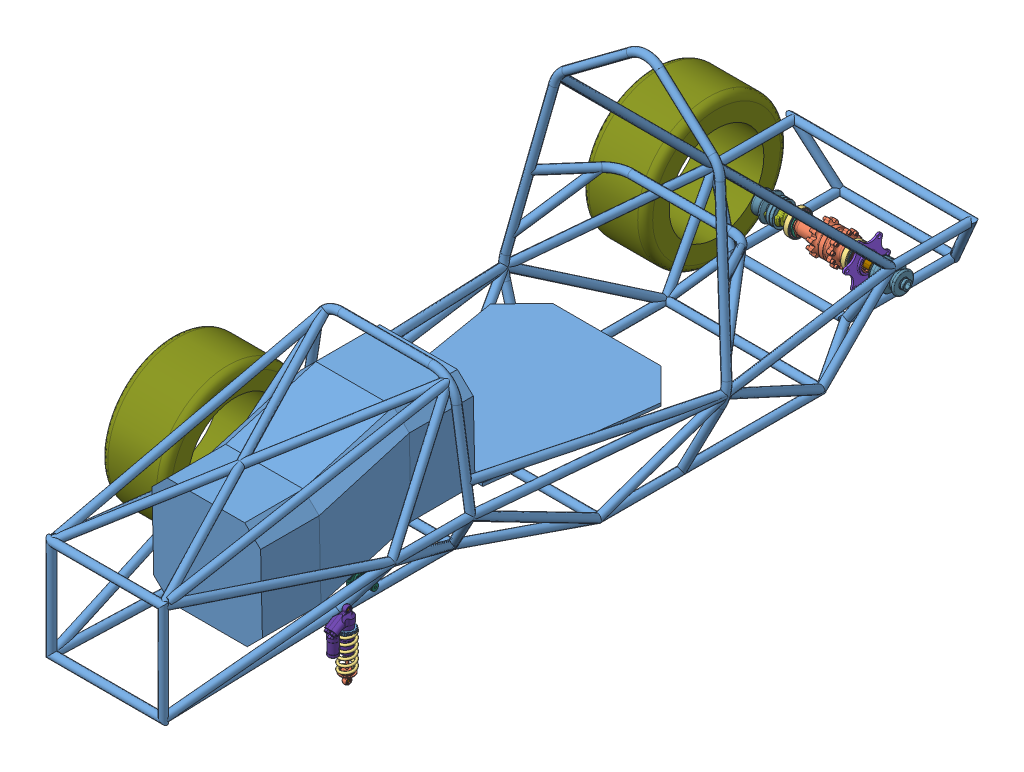
SolidWorks assembly ASSEM_Suspension24_RevA, configuration Default. Lengths in mm.
Overall size (982.83 1093.27 2583.29).
268 component instances, 21 part files, 10 mates.
Components (placement in the parent):
- 2024_Chassis_V1_RevA-1: 2024_Chassis_V1_RevA [Default<As Machined>] at origin size (743.23 992.29 2569.32)
- Differential Assembly-1: Differential Assembly [Default] at (-98.7457 437.9567 -745.2888) x (1 0 0) z (0 -0.960953 -0.276711) size (486.11 199.53 196.01)
  - Drexler Differential-1: Drexler Differential [Default] at (98.7457 177.1174 168.5551) x (0 0.999802 -0.019913) z (0 0.019913 0.999802) size (100 234.25 100)
  - SKF_32010 X-1: SKF_32010 X [Default] at (175.1207 177.1174 168.5551) x (-1 0 0) z (0 -0.454274 -0.890862) size (21.27 80 80)
    - 32010 X_or-1: 32010 X_or [Default] x (1 0 0) z (0 0 -1) size (15.5 80 80)
    - 32010 X_r-1: 32010 X_r [Default] x (1 0 0) z (0 -0.24869 -0.968583) size (15.81 10.45 7.5)
    - 32010 X_r-2: 32010 X_r [Default] x (1 0 0) z (0 -0.481754 -0.876307) size (15.81 10.45 7.5)
    - 32010 X_r-3: 32010 X_r [Default] x (1 0 0) z (0 -0.684547 -0.728969) size (15.81 10.45 7.5)
    - 32010 X_r-4: 32010 X_r [Default] x (1 0 0) z (0 -0.844328 -0.535827) size (15.81 10.45 7.5)
    - 32010 X_r-5: 32010 X_r [Default] x (1 0 0) z (0 -0.951057 -0.309017) size (15.81 10.45 7.5)
    - 32010 X_r-6: 32010 X_r [Default] x (1 0 0) z (0 -0.998027 -0.062791) size (15.81 10.45 7.5)
    - 32010 X_r-7: 32010 X_r [Default] x (1 0 0) z (0 -0.982287 0.187381) size (15.81 10.45 7.5)
    - 32010 X_r-8: 32010 X_r [Default] x (1 0 0) z (0 -0.904827 0.425779) size (15.81 10.45 7.5)
    - 32010 X_r-9: 32010 X_r [Default] x (1 0 0) z (0 -0.770513 0.637424) size (15.81 10.45 7.5)
    - 32010 X_r-10: 32010 X_r [Default] x (1 0 0) z (0 -0.587785 0.809017) size (15.81 10.45 7.5)
    - 32010 X_r-11: 32010 X_r [Default] x (1 0 0) z (0 -0.368125 0.929776) size (15.81 10.45 7.5)
    - 32010 X_r-12: 32010 X_r [Default] x (1 0 0) z (0 -0.125333 0.992115) size (15.81 10.45 7.5)
    - 32010 X_r-13: 32010 X_r [Default] x (1 0 0) z (0 0.125333 0.992115) size (15.81 10.45 7.5)
    - 32010 X_r-14: 32010 X_r [Default] x (1 0 0) z (0 0.368125 0.929776) size (15.81 10.45 7.5)
    - 32010 X_r-15: 32010 X_r [Default] x (1 0 0) z (0 0.587785 0.809017) size (15.81 10.45 7.5)
    - 32010 X_r-16: 32010 X_r [Default] x (1 0 0) z (0 0.770513 0.637424) size (15.81 10.45 7.5)
    - 32010 X_r-17: 32010 X_r [Default] x (1 0 0) z (0 0.904827 0.425779) size (15.81 10.45 7.5)
    - 32010 X_r-18: 32010 X_r [Default] x (1 0 0) z (0 0.982287 0.187381) size (15.81 10.45 7.5)
    - 32010 X_r-19: 32010 X_r [Default] x (1 0 0) z (0 0.998027 -0.062791) size (15.81 10.45 7.5)
    - 32010 X_r-20: 32010 X_r [Default] x (1 0 0) z (0 0.951057 -0.309017) size (15.81 10.45 7.5)
    - 32010 X_r-21: 32010 X_r [Default] x (1 0 0) z (0 0.844328 -0.535827) size (15.81 10.45 7.5)
    - 32010 X_r-22: 32010 X_r [Default] x (1 0 0) z (0 0.684547 -0.728969) size (15.81 10.45 7.5)
    - 32010 X_r-23: 32010 X_r [Default] x (1 0 0) z (0 0.481754 -0.876307) size (15.81 10.45 7.5)
    - 32010 X_r-24: 32010 X_r [Default] x (1 0 0) z (0 0.24869 -0.968583) size (15.81 10.45 7.5)
    - 32010 X_r-25: 32010 X_r [Default] x (1 0 0) z (0 0 -1) size (15.81 10.45 7.5)
    - 32010 X_cage-1: 32010 X_cage [Default] x (1 0 0) z (0 0 -1) size (18.02 76.15 76.15)
    - 32010 X_ir-1: 32010 X_ir [Default] x (1 0 0) z (0 0 -1) size (20 65.95 65.95)
  - SKF_32010 X-2: SKF_32010 X [Default] at (-24.8793 177.1174 168.5551) x (1 0 0) z (0 0.890912 0.454177) size (21.27 80 80)
    - 32010 X_or-1: 32010 X_or [Default] x (1 0 0) z (0 0 -1) size (15.5 80 80)
    - 32010 X_r-1: 32010 X_r [Default] x (1 0 0) z (0 -0.24869 -0.968583) size (15.81 10.45 7.5)
    - 32010 X_r-2: 32010 X_r [Default] x (1 0 0) z (0 -0.481754 -0.876307) size (15.81 10.45 7.5)
    - 32010 X_r-3: 32010 X_r [Default] x (1 0 0) z (0 -0.684547 -0.728969) size (15.81 10.45 7.5)
    - 32010 X_r-4: 32010 X_r [Default] x (1 0 0) z (0 -0.844328 -0.535827) size (15.81 10.45 7.5)
    - 32010 X_r-5: 32010 X_r [Default] x (1 0 0) z (0 -0.951057 -0.309017) size (15.81 10.45 7.5)
    - 32010 X_r-6: 32010 X_r [Default] x (1 0 0) z (0 -0.998027 -0.062791) size (15.81 10.45 7.5)
    - 32010 X_r-7: 32010 X_r [Default] x (1 0 0) z (0 -0.982287 0.187381) size (15.81 10.45 7.5)
    - 32010 X_r-8: 32010 X_r [Default] x (1 0 0) z (0 -0.904827 0.425779) size (15.81 10.45 7.5)
    - 32010 X_r-9: 32010 X_r [Default] x (1 0 0) z (0 -0.770513 0.637424) size (15.81 10.45 7.5)
    - 32010 X_r-10: 32010 X_r [Default] x (1 0 0) z (0 -0.587785 0.809017) size (15.81 10.45 7.5)
    - 32010 X_r-11: 32010 X_r [Default] x (1 0 0) z (0 -0.368125 0.929776) size (15.81 10.45 7.5)
    - 32010 X_r-12: 32010 X_r [Default] x (1 0 0) z (0 -0.125333 0.992115) size (15.81 10.45 7.5)
    - 32010 X_r-13: 32010 X_r [Default] x (1 0 0) z (0 0.125333 0.992115) size (15.81 10.45 7.5)
    - 32010 X_r-14: 32010 X_r [Default] x (1 0 0) z (0 0.368125 0.929776) size (15.81 10.45 7.5)
    - 32010 X_r-15: 32010 X_r [Default] x (1 0 0) z (0 0.587785 0.809017) size (15.81 10.45 7.5)
    - 32010 X_r-16: 32010 X_r [Default] x (1 0 0) z (0 0.770513 0.637424) size (15.81 10.45 7.5)
    - 32010 X_r-17: 32010 X_r [Default] x (1 0 0) z (0 0.904827 0.425779) size (15.81 10.45 7.5)
    - 32010 X_r-18: 32010 X_r [Default] x (1 0 0) z (0 0.982287 0.187381) size (15.81 10.45 7.5)
    - 32010 X_r-19: 32010 X_r [Default] x (1 0 0) z (0 0.998027 -0.062791) size (15.81 10.45 7.5)
    - 32010 X_r-20: 32010 X_r [Default] x (1 0 0) z (0 0.951057 -0.309017) size (15.81 10.45 7.5)
    - 32010 X_r-21: 32010 X_r [Default] x (1 0 0) z (0 0.844328 -0.535827) size (15.81 10.45 7.5)
    - 32010 X_r-22: 32010 X_r [Default] x (1 0 0) z (0 0.684547 -0.728969) size (15.81 10.45 7.5)
    - 32010 X_r-23: 32010 X_r [Default] x (1 0 0) z (0 0.481754 -0.876307) size (15.81 10.45 7.5)
    - 32010 X_r-24: 32010 X_r [Default] x (1 0 0) z (0 0.24869 -0.968583) size (15.81 10.45 7.5)
    - 32010 X_r-25: 32010 X_r [Default] x (1 0 0) z (0 0 -1) size (15.81 10.45 7.5)
    - 32010 X_cage-1: 32010 X_cage [Default] x (1 0 0) z (0 0 -1) size (18.02 76.15 76.15)
    - 32010 X_ir-1: 32010 X_ir [Default] x (1 0 0) z (0 0 -1) size (20 65.95 65.95)
  - D4825 (Drexler Long Tripod Housing)-1: D4825 (Drexler Long Tripod Housing) [Default] at (63.1207 177.1174 168.5551) x (0 0.049326 -0.998783) z (-1 0 0) size (65.36 60.36 166.5)
  - SPIDER_DIFFERENTIAL_ADAPTER-1: SPIDER_DIFFERENTIAL_ADAPTER [Default] at (197.8207 177.0374 168.5892) x (0 -0.59882 0.800884) z (-1 0 0) size (132.58 150 27.1)
  - D4824 (Drexler Medium tripod Housing)-1: D4824 (Drexler Medium tripod Housing) [Default] at (134.3707 177.1174 168.5551) x (0 0.677852 0.735198) z (1 0 0) size (65.36 60.36 155.07)
  - D4672-TA (Tripod)-1: D4672-TA (Tripod) [Default] at (321.1307 160.1151 157.3971) x (1 0 0) z (0 0.676209 0.73671) size (25.48 50.64 55.63)
    - D4672-TA.STEP-1: D4672-TA.STEP [Default] at origin size (25.48 50.64 55.63)
      - FSAE Tripod V2.STEP-1: FSAE Tripod V2.STEP [Default] at (-43.6945 4.946 19.6967) size (24.01 46.11 52.87)
      - FSAE roller_2451.STEP-1: FSAE roller_2451.STEP [Default] at (-43.6945 -7.4365 -1.7504) x (0 0.5 0.866025) z (-1 0 0) size (8.74 25.48 25.48)
      - FSAE roller_2451.STEP-2: FSAE roller_2451.STEP [Default] at (-43.6945 -7.4365 41.1438) x (0 0.5 -0.866025) z (1 0 0) size (8.74 25.48 25.48)
      - FSAE roller_2451.STEP-3: FSAE roller_2451.STEP [Default] at (-43.6945 29.711 19.6967) x (0 -1 0) z (-1 0 0) size (8.74 25.48 25.48)
      - needle.STEP-1: needle.STEP [Default] at (-42.3538 -7.5483 -1.6859) x (1 0 0) z (0 0.5 0.866025) size (1.5 1.5 10.16)
      - needle.STEP-2: needle.STEP [Default] at (-42.3574 -7.2961 -1.8314) x (0.976635 0.186114 -0.107453) z (0 0.5 0.866025) size (1.5 1.5 10.16)
      - needle.STEP-3: needle.STEP [Default] at (-42.4235 -7.0506 -1.9732) x (0.907631 0.363531 -0.209884) z (0 0.5 0.866025) size (1.5 1.5 10.16)
      - needle.STEP-4: needle.STEP [Default] at (-42.5489 -6.823 -2.1046) x (0.796213 0.523959 -0.302508) z (0 0.5 0.866025) size (1.5 1.5 10.16)
      - needle.STEP-5: needle.STEP [Default] at (-42.7279 -6.6242 -2.2194) x (0.647588 0.659903 -0.380995) z (0 0.5 0.866025) size (1.5 1.5 10.16)
      - needle.STEP-6: needle.STEP [Default] at (-42.9521 -6.4632 -2.3123) x (0.468701 0.76501 -0.441678) z (0 0.5 0.866025) size (1.5 1.5 10.16)
      - needle.STEP-7: needle.STEP [Default] at (-43.2109 -6.3478 -2.3789) x (0.267911 0.834367 -0.481722) z (0 0.5 0.866025) size (1.5 1.5 10.16)
      - needle.STEP-8: needle.STEP [Default] at (-43.4924 -6.2833 -2.4162) x (0.054602 0.864733 -0.499254) z (0 0.5 0.866025) size (1.5 1.5 10.16)
      - needle.STEP-9: needle.STEP [Default] at (-43.7833 -6.2726 -2.4224) x (-0.161259 0.854691 -0.493456) z (0 0.5 0.866025) size (1.5 1.5 10.16)
      - needle.STEP-10: needle.STEP [Default] at (-44.07 -6.3163 -2.3971) x (-0.369585 0.804708 -0.464599) z (0 0.5 0.866025) size (1.5 1.5 10.16)
      - needle.STEP-11: needle.STEP [Default] at (-44.3392 -6.4124 -2.3417) x (-0.560639 0.717121 -0.41403) z (0 0.5 0.866025) size (1.5 1.5 10.16)
      - needle.STEP-12: needle.STEP [Default] at (-44.5783 -6.5563 -2.2586) x (-0.725495 0.596023 -0.344114) z (0 0.5 0.866025) size (1.5 1.5 10.16)
      - needle.STEP-13: needle.STEP [Default] at (-44.7761 -6.7413 -2.1517) x (-0.856447 0.447072 -0.258117) z (0 0.5 0.866025) size (1.5 1.5 10.16)
      - needle.STEP-14: needle.STEP [Default] at (-44.9233 -6.9589 -2.0261) x (-0.947378 0.277229 -0.160058) z (0 0.5 0.866025) size (1.5 1.5 10.16)
      - needle.STEP-15: needle.STEP [Default] at (-45.0131 -7.1987 -1.8877) x (-0.994037 0.094432 -0.05452) z (0 0.5 0.866025) size (1.5 1.5 10.16)
      - needle.STEP-16: needle.STEP [Default] at (-45.0413 -7.4497 -1.7428) x (-0.994245 -0.092779 0.053566) z (0 0.5 0.866025) size (1.5 1.5 10.16)
      - needle.STEP-17: needle.STEP [Default] at (-45.0065 -7.7 -1.5982) x (-0.947991 -0.275654 0.159149) z (0 0.5 0.866025) size (1.5 1.5 10.16)
      - needle.STEP-18: needle.STEP [Default] at (-44.9105 -7.9381 -1.4608) x (-0.857437 -0.445647 0.257295) z (0 0.5 0.866025) size (1.5 1.5 10.16)
      - needle.STEP-19: needle.STEP [Default] at (-44.7576 -8.1527 -1.3369) x (-0.726814 -0.594816 0.343417) z (0 0.5 0.866025) size (1.5 1.5 10.16)
      - needle.STEP-20: needle.STEP [Default] at (-44.555 -8.3338 -1.2323) x (-0.562228 -0.716188 0.413491) z (0 0.5 0.866025) size (1.5 1.5 10.16)
      - needle.STEP-21: needle.STEP [Default] at (-44.3122 -8.473 -1.152) x (-0.371368 -0.804092 0.464243) z (0 0.5 0.866025) size (1.5 1.5 10.16)
      - needle.STEP-22: needle.STEP [Default] at (-44.0406 -8.5637 -1.0996) x (-0.163154 -0.854421 0.4933) z (0 0.5 0.866025) size (1.5 1.5 10.16)
      - needle.STEP-23: needle.STEP [Default] at (-43.7528 -8.6018 -1.0776) x (0.052685 -0.864823 0.499306) z (0 0.5 0.866025) size (1.5 1.5 10.16)
      - needle.STEP-24: needle.STEP [Default] at (-43.4622 -8.5854 -1.0871) x (0.266061 -0.834811 0.481978) z (0 0.5 0.866025) size (1.5 1.5 10.16)
      - needle.STEP-25: needle.STEP [Default] at (-43.1825 -8.5153 -1.1275) x (0.467004 -0.765787 0.442128) z (0 0.5 0.866025) size (1.5 1.5 10.16)
      - needle.STEP-26: needle.STEP [Default] at (-42.9268 -8.3949 -1.1971) x (0.646124 -0.660979 0.381616) z (0 0.5 0.866025) size (1.5 1.5 10.16)
      - needle.STEP-27: needle.STEP [Default] at (-42.7069 -8.2296 -1.2925) x (0.79505 -0.525282 0.303272) z (0 0.5 0.866025) size (1.5 1.5 10.16)
      - needle.STEP-28: needle.STEP [Default] at (-42.5332 -8.0272 -1.4093) x (0.906823 -0.365039 0.210755) z (0 0.5 0.866025) size (1.5 1.5 10.16)
      - needle.STEP-29: needle.STEP [Default] at (-42.4137 -7.7973 -1.5421) x (0.97622 -0.187737 0.10839) z (0 0.5 0.866025) size (1.5 1.5 10.16)
      - needle.STEP-30: needle.STEP [Default] at (-42.3538 29.711 19.5676) x (1 0 0) z (0 -1 0) size (1.5 1.5 10.16)
      - needle.STEP-31: needle.STEP [Default] at (-42.3538 -7.3247 41.2084) x (1 0 0) z (0 0.5 -0.866025) size (1.5 1.5 10.16)
      - needle.STEP-32: needle.STEP [Default] at (-42.4137 29.711 19.2801) x (0.97622 0 -0.21678) z (0 -1 0) size (1.5 1.5 10.16)
      - needle.STEP-33: needle.STEP [Default] at (-42.4137 -7.0756 41.3522) x (0.97622 0.187737 0.10839) z (0 0.5 -0.866025) size (1.5 1.5 10.16)
      - needle.STEP-34: needle.STEP [Default] at (-42.5332 29.711 19.0146) x (0.906823 0 -0.421511) z (0 -1 0) size (1.5 1.5 10.16)
      - needle.STEP-35: needle.STEP [Default] at (-42.5332 -6.8457 41.4849) x (0.906823 0.365039 0.210755) z (0 0.5 -0.866025) size (1.5 1.5 10.16)
      - needle.STEP-36: needle.STEP [Default] at (-42.7069 29.711 18.7809) x (0.79505 0 -0.606544) z (0 -1 0) size (1.5 1.5 10.16)
      - needle.STEP-37: needle.STEP [Default] at (-42.7069 -6.6434 41.6017) x (0.79505 0.525282 0.303272) z (0 0.5 -0.866025) size (1.5 1.5 10.16)
      - needle.STEP-38: needle.STEP [Default] at (-42.9268 29.711 18.5901) x (0.646124 0 -0.763232) z (0 -1 0) size (1.5 1.5 10.16)
      - needle.STEP-39: needle.STEP [Default] at (-42.9268 -6.4781 41.6972) x (0.646124 0.660979 0.381616) z (0 0.5 -0.866025) size (1.5 1.5 10.16)
      - needle.STEP-40: needle.STEP [Default] at (-43.1825 29.711 18.4509) x (0.467004 0 -0.884255) z (0 -1 0) size (1.5 1.5 10.16)
      - needle.STEP-41: needle.STEP [Default] at (-43.1825 -6.3576 41.7667) x (0.467004 0.765787 0.442128) z (0 0.5 -0.866025) size (1.5 1.5 10.16)
      - needle.STEP-42: needle.STEP [Default] at (-43.4622 29.711 18.37) x (0.266061 0 -0.963956) z (0 -1 0) size (1.5 1.5 10.16)
      - needle.STEP-43: needle.STEP [Default] at (-43.4622 -6.2875 41.8072) x (0.266061 0.834811 0.481978) z (0 0.5 -0.866025) size (1.5 1.5 10.16)
      - needle.STEP-44: needle.STEP [Default] at (-43.7528 29.711 18.3511) x (0.052685 0 -0.998611) z (0 -1 0) size (1.5 1.5 10.16)
      - needle.STEP-45: needle.STEP [Default] at (-43.7528 -6.2711 41.8166) x (0.052685 0.864823 0.499306) z (0 0.5 -0.866025) size (1.5 1.5 10.16)
      - needle.STEP-46: needle.STEP [Default] at (-44.0406 29.711 18.3951) x (-0.163154 0 -0.986601) z (0 -1 0) size (1.5 1.5 10.16)
      - needle.STEP-47: needle.STEP [Default] at (-44.0406 -6.3092 41.7947) x (-0.163154 0.854421 0.4933) z (0 0.5 -0.866025) size (1.5 1.5 10.16)
      - needle.STEP-48: needle.STEP [Default] at (-44.3122 29.711 18.4999) x (-0.371368 0 -0.928486) z (0 -1 0) size (1.5 1.5 10.16)
      - needle.STEP-49: needle.STEP [Default] at (-44.3122 -6.4 41.7423) x (-0.371368 0.804092 0.464243) z (0 0.5 -0.866025) size (1.5 1.5 10.16)
      - needle.STEP-50: needle.STEP [Default] at (-44.555 29.711 18.6606) x (-0.562228 0 -0.826982) z (0 -1 0) size (1.5 1.5 10.16)
      - needle.STEP-51: needle.STEP [Default] at (-44.555 -6.5392 41.6619) x (-0.562228 0.716188 0.413491) z (0 0.5 -0.866025) size (1.5 1.5 10.16)
      - needle.STEP-52: needle.STEP [Default] at (-44.7576 29.711 18.8697) x (-0.726814 0 -0.686834) z (0 -1 0) size (1.5 1.5 10.16)
      - needle.STEP-53: needle.STEP [Default] at (-44.7576 -6.7203 41.5573) x (-0.726814 0.594816 0.343417) z (0 0.5 -0.866025) size (1.5 1.5 10.16)
      - needle.STEP-54: needle.STEP [Default] at (-44.9105 29.711 19.1175) x (-0.857437 0 -0.514589) z (0 -1 0) size (1.5 1.5 10.16)
      - needle.STEP-55: needle.STEP [Default] at (-44.9105 -6.9349 41.4334) x (-0.857437 0.445647 0.257295) z (0 0.5 -0.866025) size (1.5 1.5 10.16)
      - needle.STEP-56: needle.STEP [Default] at (-45.0065 29.711 19.3924) x (-0.947991 0 -0.318298) z (0 -1 0) size (1.5 1.5 10.16)
      - needle.STEP-57: needle.STEP [Default] at (-45.0065 -7.1729 41.296) x (-0.947991 0.275654 0.159149) z (0 0.5 -0.866025) size (1.5 1.5 10.16)
      - needle.STEP-58: needle.STEP [Default] at (-45.0413 29.711 19.6814) x (-0.994245 0 -0.107132) z (0 -1 0) size (1.5 1.5 10.16)
      - needle.STEP-59: needle.STEP [Default] at (-45.0413 -7.4232 41.1515) x (-0.994245 0.092779 0.053566) z (0 0.5 -0.866025) size (1.5 1.5 10.16)
      - needle.STEP-60: needle.STEP [Default] at (-45.0131 29.711 19.9712) x (-0.994037 0 0.10904) z (0 -1 0) size (1.5 1.5 10.16)
      - needle.STEP-61: needle.STEP [Default] at (-45.0131 -7.6742 41.0066) x (-0.994037 -0.094432 -0.05452) z (0 0.5 -0.866025) size (1.5 1.5 10.16)
      - needle.STEP-62: needle.STEP [Default] at (-44.9233 29.711 20.2482) x (-0.947378 0 0.320117) z (0 -1 0) size (1.5 1.5 10.16)
      - needle.STEP-63: needle.STEP [Default] at (-44.9233 -7.914 40.8681) x (-0.947378 -0.277229 -0.160058) z (0 0.5 -0.866025) size (1.5 1.5 10.16)
      - needle.STEP-64: needle.STEP [Default] at (-44.7761 29.711 20.4994) x (-0.856447 0 0.516234) z (0 -1 0) size (1.5 1.5 10.16)
      - needle.STEP-65: needle.STEP [Default] at (-44.7761 -8.1316 40.7425) x (-0.856447 -0.447072 -0.258117) z (0 0.5 -0.866025) size (1.5 1.5 10.16)
      - needle.STEP-66: needle.STEP [Default] at (-44.5783 29.711 20.7131) x (-0.725495 0 0.688228) z (0 -1 0) size (1.5 1.5 10.16)
      - needle.STEP-67: needle.STEP [Default] at (-44.5783 -8.3166 40.6357) x (-0.725495 -0.596023 -0.344114) z (0 0.5 -0.866025) size (1.5 1.5 10.16)
      - needle.STEP-68: needle.STEP [Default] at (-44.3392 29.711 20.8792) x (-0.560639 0 0.82806) z (0 -1 0) size (1.5 1.5 10.16)
      - needle.STEP-69: needle.STEP [Default] at (-44.3392 -8.4606 40.5526) x (-0.560639 -0.717121 -0.41403) z (0 0.5 -0.866025) size (1.5 1.5 10.16)
      - needle.STEP-70: needle.STEP [Default] at (-44.07 29.711 20.9902) x (-0.369585 0 0.929197) z (0 -1 0) size (1.5 1.5 10.16)
      - needle.STEP-71: needle.STEP [Default] at (-44.07 -8.5566 40.4971) x (-0.369585 -0.804708 -0.464599) z (0 0.5 -0.866025) size (1.5 1.5 10.16)
      - needle.STEP-72: needle.STEP [Default] at (-43.7833 29.711 21.0407) x (-0.161259 0 0.986912) z (0 -1 0) size (1.5 1.5 10.16)
      - needle.STEP-73: needle.STEP [Default] at (-43.7833 -8.6003 40.4719) x (-0.161259 -0.854691 -0.493456) z (0 0.5 -0.866025) size (1.5 1.5 10.16)
      - needle.STEP-74: needle.STEP [Default] at (-43.4924 29.711 21.0283) x (0.054602 0 0.998508) z (0 -1 0) size (1.5 1.5 10.16)
      - needle.STEP-75: needle.STEP [Default] at (-43.4924 -8.5897 40.478) x (0.054602 -0.864733 -0.499254) z (0 0.5 -0.866025) size (1.5 1.5 10.16)
      - needle.STEP-76: needle.STEP [Default] at (-43.2109 29.711 20.9538) x (0.267911 0 0.963444) z (0 -1 0) size (1.5 1.5 10.16)
      - needle.STEP-77: needle.STEP [Default] at (-43.2109 -8.5251 40.5153) x (0.267911 -0.834367 -0.481722) z (0 0.5 -0.866025) size (1.5 1.5 10.16)
      - needle.STEP-78: needle.STEP [Default] at (-42.9521 29.711 20.8205) x (0.468701 0 0.883357) z (0 -1 0) size (1.5 1.5 10.16)
      - needle.STEP-79: needle.STEP [Default] at (-42.9521 -8.4097 40.582) x (0.468701 -0.76501 -0.441678) z (0 0.5 -0.866025) size (1.5 1.5 10.16)
      - needle.STEP-80: needle.STEP [Default] at (-42.7279 29.711 20.6347) x (0.647588 0 0.761991) z (0 -1 0) size (1.5 1.5 10.16)
      - needle.STEP-81: needle.STEP [Default] at (-42.7279 -8.2488 40.6749) x (0.647588 -0.659903 -0.380995) z (0 0.5 -0.866025) size (1.5 1.5 10.16)
      - needle.STEP-82: needle.STEP [Default] at (-42.5489 29.711 20.4051) x (0.796213 0 0.605016) z (0 -1 0) size (1.5 1.5 10.16)
      - needle.STEP-83: needle.STEP [Default] at (-42.5489 -8.0499 40.7897) x (0.796213 -0.523959 -0.302508) z (0 0.5 -0.866025) size (1.5 1.5 10.16)
      - needle.STEP-84: needle.STEP [Default] at (-42.4235 29.711 20.1423) x (0.907631 0 0.419769) z (0 -1 0) size (1.5 1.5 10.16)
      - needle.STEP-85: needle.STEP [Default] at (-42.4235 -7.8224 40.921) x (0.907631 -0.363531 -0.209884) z (0 0.5 -0.866025) size (1.5 1.5 10.16)
      - needle.STEP-86: needle.STEP [Default] at (-42.3574 29.711 19.8588) x (0.976635 0 0.214906) z (0 -1 0) size (1.5 1.5 10.16)
      - needle.STEP-87: needle.STEP [Default] at (-42.3574 -7.5768 41.0628) x (0.976635 -0.186114 -0.107453) z (0 0.5 -0.866025) size (1.5 1.5 10.16)
      - Tripod Retainer.STEP-1: Tripod Retainer.STEP [Default] at (-43.6945 -8.0715 -2.8502) x (0.973299 0.198788 -0.11477) z (0 0.5 0.866025) size (15.88 15.88 1.27)
      - Tripod Retainer.STEP-2: Tripod Retainer.STEP [Default] at (-43.6945 -8.0715 42.2437) x (0.973299 -0.198788 -0.11477) z (0 0.5 -0.866025) size (15.88 15.88 1.27)
      - Tripod Retainer.STEP-3: Tripod Retainer.STEP [Default] at (-43.6945 30.981 19.6967) x (0.973299 0 0.229541) z (0 -1 0) size (15.88 15.88 1.27)
  - D4672-TA (Tripod)-2: D4672-TA (Tripod) [Default] at (-47.6803 161.7899 181.8937) x (1 0 0) z (0 0.890652 -0.454686) size (25.48 50.64 55.63)
    - D4672-TA.STEP-1: D4672-TA.STEP [Default] at origin size (25.48 50.64 55.63)
      - FSAE Tripod V2.STEP-1: FSAE Tripod V2.STEP [Default] at (-43.6945 4.946 19.6967) size (24.01 46.11 52.87)
      - FSAE roller_2451.STEP-1: FSAE roller_2451.STEP [Default] at (-43.6945 -7.4365 -1.7504) x (0 0.5 0.866025) z (-1 0 0) size (8.74 25.48 25.48)
      - FSAE roller_2451.STEP-2: FSAE roller_2451.STEP [Default] at (-43.6945 -7.4365 41.1438) x (0 0.5 -0.866025) z (1 0 0) size (8.74 25.48 25.48)
      - FSAE roller_2451.STEP-3: FSAE roller_2451.STEP [Default] at (-43.6945 29.711 19.6967) x (0 -1 0) z (-1 0 0) size (8.74 25.48 25.48)
      - needle.STEP-1: needle.STEP [Default] at (-42.3538 -7.5483 -1.6859) x (1 0 0) z (0 0.5 0.866025) size (1.5 1.5 10.16)
      - needle.STEP-2: needle.STEP [Default] at (-42.3574 -7.2961 -1.8314) x (0.976635 0.186114 -0.107453) z (0 0.5 0.866025) size (1.5 1.5 10.16)
      - needle.STEP-3: needle.STEP [Default] at (-42.4235 -7.0506 -1.9732) x (0.907631 0.363531 -0.209884) z (0 0.5 0.866025) size (1.5 1.5 10.16)
      - needle.STEP-4: needle.STEP [Default] at (-42.5489 -6.823 -2.1046) x (0.796213 0.523959 -0.302508) z (0 0.5 0.866025) size (1.5 1.5 10.16)
      - needle.STEP-5: needle.STEP [Default] at (-42.7279 -6.6242 -2.2194) x (0.647588 0.659903 -0.380995) z (0 0.5 0.866025) size (1.5 1.5 10.16)
      - needle.STEP-6: needle.STEP [Default] at (-42.9521 -6.4632 -2.3123) x (0.468701 0.76501 -0.441678) z (0 0.5 0.866025) size (1.5 1.5 10.16)
      - needle.STEP-7: needle.STEP [Default] at (-43.2109 -6.3478 -2.3789) x (0.267911 0.834367 -0.481722) z (0 0.5 0.866025) size (1.5 1.5 10.16)
      - needle.STEP-8: needle.STEP [Default] at (-43.4924 -6.2833 -2.4162) x (0.054602 0.864733 -0.499254) z (0 0.5 0.866025) size (1.5 1.5 10.16)
      - needle.STEP-9: needle.STEP [Default] at (-43.7833 -6.2726 -2.4224) x (-0.161259 0.854691 -0.493456) z (0 0.5 0.866025) size (1.5 1.5 10.16)
      - needle.STEP-10: needle.STEP [Default] at (-44.07 -6.3163 -2.3971) x (-0.369585 0.804708 -0.464599) z (0 0.5 0.866025) size (1.5 1.5 10.16)
      - needle.STEP-11: needle.STEP [Default] at (-44.3392 -6.4124 -2.3417) x (-0.560639 0.717121 -0.41403) z (0 0.5 0.866025) size (1.5 1.5 10.16)
      - needle.STEP-12: needle.STEP [Default] at (-44.5783 -6.5563 -2.2586) x (-0.725495 0.596023 -0.344114) z (0 0.5 0.866025) size (1.5 1.5 10.16)
      - needle.STEP-13: needle.STEP [Default] at (-44.7761 -6.7413 -2.1517) x (-0.856447 0.447072 -0.258117) z (0 0.5 0.866025) size (1.5 1.5 10.16)
      - needle.STEP-14: needle.STEP [Default] at (-44.9233 -6.9589 -2.0261) x (-0.947378 0.277229 -0.160058) z (0 0.5 0.866025) size (1.5 1.5 10.16)
      - needle.STEP-15: needle.STEP [Default] at (-45.0131 -7.1987 -1.8877) x (-0.994037 0.094432 -0.05452) z (0 0.5 0.866025) size (1.5 1.5 10.16)
      - needle.STEP-16: needle.STEP [Default] at (-45.0413 -7.4497 -1.7428) x (-0.994245 -0.092779 0.053566) z (0 0.5 0.866025) size (1.5 1.5 10.16)
      - needle.STEP-17: needle.STEP [Default] at (-45.0065 -7.7 -1.5982) x (-0.947991 -0.275654 0.159149) z (0 0.5 0.866025) size (1.5 1.5 10.16)
      - needle.STEP-18: needle.STEP [Default] at (-44.9105 -7.9381 -1.4608) x (-0.857437 -0.445647 0.257295) z (0 0.5 0.866025) size (1.5 1.5 10.16)
      - needle.STEP-19: needle.STEP [Default] at (-44.7576 -8.1527 -1.3369) x (-0.726814 -0.594816 0.343417) z (0 0.5 0.866025) size (1.5 1.5 10.16)
      - needle.STEP-20: needle.STEP [Default] at (-44.555 -8.3338 -1.2323) x (-0.562228 -0.716188 0.413491) z (0 0.5 0.866025) size (1.5 1.5 10.16)
      - needle.STEP-21: needle.STEP [Default] at (-44.3122 -8.473 -1.152) x (-0.371368 -0.804092 0.464243) z (0 0.5 0.866025) size (1.5 1.5 10.16)
      - needle.STEP-22: needle.STEP [Default] at (-44.0406 -8.5637 -1.0996) x (-0.163154 -0.854421 0.4933) z (0 0.5 0.866025) size (1.5 1.5 10.16)
      - needle.STEP-23: needle.STEP [Default] at (-43.7528 -8.6018 -1.0776) x (0.052685 -0.864823 0.499306) z (0 0.5 0.866025) size (1.5 1.5 10.16)
      - needle.STEP-24: needle.STEP [Default] at (-43.4622 -8.5854 -1.0871) x (0.266061 -0.834811 0.481978) z (0 0.5 0.866025) size (1.5 1.5 10.16)
      - needle.STEP-25: needle.STEP [Default] at (-43.1825 -8.5153 -1.1275) x (0.467004 -0.765787 0.442128) z (0 0.5 0.866025) size (1.5 1.5 10.16)
      - needle.STEP-26: needle.STEP [Default] at (-42.9268 -8.3949 -1.1971) x (0.646124 -0.660979 0.381616) z (0 0.5 0.866025) size (1.5 1.5 10.16)
      - needle.STEP-27: needle.STEP [Default] at (-42.7069 -8.2296 -1.2925) x (0.79505 -0.525282 0.303272) z (0 0.5 0.866025) size (1.5 1.5 10.16)
      - needle.STEP-28: needle.STEP [Default] at (-42.5332 -8.0272 -1.4093) x (0.906823 -0.365039 0.210755) z (0 0.5 0.866025) size (1.5 1.5 10.16)
      - needle.STEP-29: needle.STEP [Default] at (-42.4137 -7.7973 -1.5421) x (0.97622 -0.187737 0.10839) z (0 0.5 0.866025) size (1.5 1.5 10.16)
      - needle.STEP-30: needle.STEP [Default] at (-42.3538 29.711 19.5676) x (1 0 0) z (0 -1 0) size (1.5 1.5 10.16)
      - needle.STEP-31: needle.STEP [Default] at (-42.3538 -7.3247 41.2084) x (1 0 0) z (0 0.5 -0.866025) size (1.5 1.5 10.16)
      - needle.STEP-32: needle.STEP [Default] at (-42.4137 29.711 19.2801) x (0.97622 0 -0.21678) z (0 -1 0) size (1.5 1.5 10.16)
      - needle.STEP-33: needle.STEP [Default] at (-42.4137 -7.0756 41.3522) x (0.97622 0.187737 0.10839) z (0 0.5 -0.866025) size (1.5 1.5 10.16)
      - needle.STEP-34: needle.STEP [Default] at (-42.5332 29.711 19.0146) x (0.906823 0 -0.421511) z (0 -1 0) size (1.5 1.5 10.16)
      - needle.STEP-35: needle.STEP [Default] at (-42.5332 -6.8457 41.4849) x (0.906823 0.365039 0.210755) z (0 0.5 -0.866025) size (1.5 1.5 10.16)
      - needle.STEP-36: needle.STEP [Default] at (-42.7069 29.711 18.7809) x (0.79505 0 -0.606544) z (0 -1 0) size (1.5 1.5 10.16)
      - needle.STEP-37: needle.STEP [Default] at (-42.7069 -6.6434 41.6017) x (0.79505 0.525282 0.303272) z (0 0.5 -0.866025) size (1.5 1.5 10.16)
      - needle.STEP-38: needle.STEP [Default] at (-42.9268 29.711 18.5901) x (0.646124 0 -0.763232) z (0 -1 0) size (1.5 1.5 10.16)
      - needle.STEP-39: needle.STEP [Default] at (-42.9268 -6.4781 41.6972) x (0.646124 0.660979 0.381616) z (0 0.5 -0.866025) size (1.5 1.5 10.16)
      - needle.STEP-40: needle.STEP [Default] at (-43.1825 29.711 18.4509) x (0.467004 0 -0.884255) z (0 -1 0) size (1.5 1.5 10.16)
      - needle.STEP-41: needle.STEP [Default] at (-43.1825 -6.3576 41.7667) x (0.467004 0.765787 0.442128) z (0 0.5 -0.866025) size (1.5 1.5 10.16)
      - needle.STEP-42: needle.STEP [Default] at (-43.4622 29.711 18.37) x (0.266061 0 -0.963956) z (0 -1 0) size (1.5 1.5 10.16)
      - needle.STEP-43: needle.STEP [Default] at (-43.4622 -6.2875 41.8072) x (0.266061 0.834811 0.481978) z (0 0.5 -0.866025) size (1.5 1.5 10.16)
      - needle.STEP-44: needle.STEP [Default] at (-43.7528 29.711 18.3511) x (0.052685 0 -0.998611) z (0 -1 0) size (1.5 1.5 10.16)
      - needle.STEP-45: needle.STEP [Default] at (-43.7528 -6.2711 41.8166) x (0.052685 0.864823 0.499306) z (0 0.5 -0.866025) size (1.5 1.5 10.16)
      - needle.STEP-46: needle.STEP [Default] at (-44.0406 29.711 18.3951) x (-0.163154 0 -0.986601) z (0 -1 0) size (1.5 1.5 10.16)
      - needle.STEP-47: needle.STEP [Default] at (-44.0406 -6.3092 41.7947) x (-0.163154 0.854421 0.4933) z (0 0.5 -0.866025) size (1.5 1.5 10.16)
      - needle.STEP-48: needle.STEP [Default] at (-44.3122 29.711 18.4999) x (-0.371368 0 -0.928486) z (0 -1 0) size (1.5 1.5 10.16)
      - needle.STEP-49: needle.STEP [Default] at (-44.3122 -6.4 41.7423) x (-0.371368 0.804092 0.464243) z (0 0.5 -0.866025) size (1.5 1.5 10.16)
      - needle.STEP-50: needle.STEP [Default] at (-44.555 29.711 18.6606) x (-0.562228 0 -0.826982) z (0 -1 0) size (1.5 1.5 10.16)
      - needle.STEP-51: needle.STEP [Default] at (-44.555 -6.5392 41.6619) x (-0.562228 0.716188 0.413491) z (0 0.5 -0.866025) size (1.5 1.5 10.16)
      - needle.STEP-52: needle.STEP [Default] at (-44.7576 29.711 18.8697) x (-0.726814 0 -0.686834) z (0 -1 0) size (1.5 1.5 10.16)
      - needle.STEP-53: needle.STEP [Default] at (-44.7576 -6.7203 41.5573) x (-0.726814 0.594816 0.343417) z (0 0.5 -0.866025) size (1.5 1.5 10.16)
      - needle.STEP-54: needle.STEP [Default] at (-44.9105 29.711 19.1175) x (-0.857437 0 -0.514589) z (0 -1 0) size (1.5 1.5 10.16)
      - needle.STEP-55: needle.STEP [Default] at (-44.9105 -6.9349 41.4334) x (-0.857437 0.445647 0.257295) z (0 0.5 -0.866025) size (1.5 1.5 10.16)
      - needle.STEP-56: needle.STEP [Default] at (-45.0065 29.711 19.3924) x (-0.947991 0 -0.318298) z (0 -1 0) size (1.5 1.5 10.16)
      - needle.STEP-57: needle.STEP [Default] at (-45.0065 -7.1729 41.296) x (-0.947991 0.275654 0.159149) z (0 0.5 -0.866025) size (1.5 1.5 10.16)
      - needle.STEP-58: needle.STEP [Default] at (-45.0413 29.711 19.6814) x (-0.994245 0 -0.107132) z (0 -1 0) size (1.5 1.5 10.16)
      - needle.STEP-59: needle.STEP [Default] at (-45.0413 -7.4232 41.1515) x (-0.994245 0.092779 0.053566) z (0 0.5 -0.866025) size (1.5 1.5 10.16)
      - needle.STEP-60: needle.STEP [Default] at (-45.0131 29.711 19.9712) x (-0.994037 0 0.10904) z (0 -1 0) size (1.5 1.5 10.16)
      - needle.STEP-61: needle.STEP [Default] at (-45.0131 -7.6742 41.0066) x (-0.994037 -0.094432 -0.05452) z (0 0.5 -0.866025) size (1.5 1.5 10.16)
      - needle.STEP-62: needle.STEP [Default] at (-44.9233 29.711 20.2482) x (-0.947378 0 0.320117) z (0 -1 0) size (1.5 1.5 10.16)
      - needle.STEP-63: needle.STEP [Default] at (-44.9233 -7.914 40.8681) x (-0.947378 -0.277229 -0.160058) z (0 0.5 -0.866025) size (1.5 1.5 10.16)
      - needle.STEP-64: needle.STEP [Default] at (-44.7761 29.711 20.4994) x (-0.856447 0 0.516234) z (0 -1 0) size (1.5 1.5 10.16)
      - needle.STEP-65: needle.STEP [Default] at (-44.7761 -8.1316 40.7425) x (-0.856447 -0.447072 -0.258117) z (0 0.5 -0.866025) size (1.5 1.5 10.16)
      - needle.STEP-66: needle.STEP [Default] at (-44.5783 29.711 20.7131) x (-0.725495 0 0.688228) z (0 -1 0) size (1.5 1.5 10.16)
      - needle.STEP-67: needle.STEP [Default] at (-44.5783 -8.3166 40.6357) x (-0.725495 -0.596023 -0.344114) z (0 0.5 -0.866025) size (1.5 1.5 10.16)
      - needle.STEP-68: needle.STEP [Default] at (-44.3392 29.711 20.8792) x (-0.560639 0 0.82806) z (0 -1 0) size (1.5 1.5 10.16)
      - needle.STEP-69: needle.STEP [Default] at (-44.3392 -8.4606 40.5526) x (-0.560639 -0.717121 -0.41403) z (0 0.5 -0.866025) size (1.5 1.5 10.16)
      - needle.STEP-70: needle.STEP [Default] at (-44.07 29.711 20.9902) x (-0.369585 0 0.929197) z (0 -1 0) size (1.5 1.5 10.16)
      - needle.STEP-71: needle.STEP [Default] at (-44.07 -8.5566 40.4971) x (-0.369585 -0.804708 -0.464599) z (0 0.5 -0.866025) size (1.5 1.5 10.16)
      - needle.STEP-72: needle.STEP [Default] at (-43.7833 29.711 21.0407) x (-0.161259 0 0.986912) z (0 -1 0) size (1.5 1.5 10.16)
      - needle.STEP-73: needle.STEP [Default] at (-43.7833 -8.6003 40.4719) x (-0.161259 -0.854691 -0.493456) z (0 0.5 -0.866025) size (1.5 1.5 10.16)
      - needle.STEP-74: needle.STEP [Default] at (-43.4924 29.711 21.0283) x (0.054602 0 0.998508) z (0 -1 0) size (1.5 1.5 10.16)
      - needle.STEP-75: needle.STEP [Default] at (-43.4924 -8.5897 40.478) x (0.054602 -0.864733 -0.499254) z (0 0.5 -0.866025) size (1.5 1.5 10.16)
      - needle.STEP-76: needle.STEP [Default] at (-43.2109 29.711 20.9538) x (0.267911 0 0.963444) z (0 -1 0) size (1.5 1.5 10.16)
      - needle.STEP-77: needle.STEP [Default] at (-43.2109 -8.5251 40.5153) x (0.267911 -0.834367 -0.481722) z (0 0.5 -0.866025) size (1.5 1.5 10.16)
      - needle.STEP-78: needle.STEP [Default] at (-42.9521 29.711 20.8205) x (0.468701 0 0.883357) z (0 -1 0) size (1.5 1.5 10.16)
      - needle.STEP-79: needle.STEP [Default] at (-42.9521 -8.4097 40.582) x (0.468701 -0.76501 -0.441678) z (0 0.5 -0.866025) size (1.5 1.5 10.16)
      - needle.STEP-80: needle.STEP [Default] at (-42.7279 29.711 20.6347) x (0.647588 0 0.761991) z (0 -1 0) size (1.5 1.5 10.16)
      - needle.STEP-81: needle.STEP [Default] at (-42.7279 -8.2488 40.6749) x (0.647588 -0.659903 -0.380995) z (0 0.5 -0.866025) size (1.5 1.5 10.16)
      - needle.STEP-82: needle.STEP [Default] at (-42.5489 29.711 20.4051) x (0.796213 0 0.605016) z (0 -1 0) size (1.5 1.5 10.16)
      - needle.STEP-83: needle.STEP [Default] at (-42.5489 -8.0499 40.7897) x (0.796213 -0.523959 -0.302508) z (0 0.5 -0.866025) size (1.5 1.5 10.16)
      - needle.STEP-84: needle.STEP [Default] at (-42.4235 29.711 20.1423) x (0.907631 0 0.419769) z (0 -1 0) size (1.5 1.5 10.16)
      - needle.STEP-85: needle.STEP [Default] at (-42.4235 -7.8224 40.921) x (0.907631 -0.363531 -0.209884) z (0 0.5 -0.866025) size (1.5 1.5 10.16)
      - needle.STEP-86: needle.STEP [Default] at (-42.3574 29.711 19.8588) x (0.976635 0 0.214906) z (0 -1 0) size (1.5 1.5 10.16)
      - needle.STEP-87: needle.STEP [Default] at (-42.3574 -7.5768 41.0628) x (0.976635 -0.186114 -0.107453) z (0 0.5 -0.866025) size (1.5 1.5 10.16)
      - Tripod Retainer.STEP-1: Tripod Retainer.STEP [Default] at (-43.6945 -8.0715 -2.8502) x (0.973299 0.198788 -0.11477) z (0 0.5 0.866025) size (15.88 15.88 1.27)
      - Tripod Retainer.STEP-2: Tripod Retainer.STEP [Default] at (-43.6945 -8.0715 42.2437) x (0.973299 -0.198788 -0.11477) z (0 0.5 -0.866025) size (15.88 15.88 1.27)
      - Tripod Retainer.STEP-3: Tripod Retainer.STEP [Default] at (-43.6945 30.981 19.6967) x (0.973299 0 0.229541) z (0 -1 0) size (15.88 15.88 1.27)
  - 615-3 (Triangular Tripod Housing Boot)-1: 615-3 (Triangular Tripod Housing Boot) [Default] at (336.0855 177.1174 168.5551) x (0 0.694966 -0.719043) z (1 0 0) size (84.51 84.51 88.49)
  - 615-3 (Triangular Tripod Housing Boot)-2: 615-3 (Triangular Tripod Housing Boot) [Default] at (-150.024 177.1174 168.5551) x (0 -0.881387 -0.472395) z (-1 0 0) size (84.51 84.51 88.49)
- KAZ_Steering_Rack_-_Dumb_Solid-1: KAZ_Steering_Rack_-_Dumb_Solid [Default] at (0 198.8947 1049.6828) x (1 0 0) z (0 1 0) size (386.71 91.39 96.37)
- HoosierTyres_43100Slicks-1: HoosierTyres_43100Slicks [Default] at (-403.86 204.47 902.2716) x (0 1 0) z (0 0 1) size (459.74 205.74 459.74)
- HoosierTyres_43100Slicks-2: HoosierTyres_43100Slicks [Default] at (-378.46 204.47 -621.7284) x (0 -1 0) z (0 0 -1) size (459.74 205.74 459.74)
- Ohlins TTX25 Shock 50mm-1: Ohlins TTX25 Shock 50mm [Default] at (193.4522 185.0928 1140.6054) size (68.2 222.5 95.1)
  - Body-1: Body [Default] at origin size (40.15 132 80.5)
  - M8 ball-1: M8 ball [Default] x (0 0 -1) z (1 0 0) size (12.5 12.5 8)
  - M8 ball-2: M8 ball [Default] at (0 -199.5 0) x (0 0 -1) z (1 0 0) size (12.5 12.5 8)
  - Tightening nut-1: Tightening nut [Default] at (0 -4 0) x (-0.593403 0 0.804906) z (-0.804906 0 -0.593403) size (48.77 20 48.77)
  - Piston-1: Piston [Default] at (0 0.13 0) x (-0.999632 0 -0.027131) z (0.027131 0 -0.999632) size (46 115.5 45.56)
  - Spring-1: Spring [Default] at (0 -176 0) size (54.68 133 54.06)
Mates (geometry in assembly coordinates):
- Concentric1: concentric anti-aligned: cylinder of Differential Assembly-1/Drexler Differential-1 through (-121.625 226.9728 -621.7284) axis (1 0 0) radius 25
- Coincident2: coincident: point of Differential Assembly-1/Drexler Differential-1
- Coincident4: coincident anti-aligned: plane of KAZ_Steering_Rack_-_Dumb_Solid-1 through (139.7 173.4947 1079.6167) normal (0 -1 0)
- Coincident5: coincident anti-aligned: plane of KAZ_Steering_Rack_-_Dumb_Solid-1 through (0 198.8947 1049.6828) normal (-1 0 0)
- Tangent1: tangent anti-aligned: cylinder of HoosierTyres_43100Slicks-1 through (-403.86 204.47 902.2716) axis (1 0 0) radius 229.87
- Tangent2: tangent anti-aligned: cylinder of HoosierTyres_43100Slicks-2 through (-378.46 204.47 -621.7284) axis (1 0 0) radius 229.87
- Distance1: distance = 25.4 mm aligned: plane of HoosierTyres_43100Slicks-1 through (-609.6 52.07 902.2716) normal (-1 0 0); plane of HoosierTyres_43100Slicks-2 through (-584.2 356.87 -621.7284) normal (-1 0 0)
- Coincident8: coincident anti-aligned: plane of HoosierTyres_43100Slicks-1 through (-403.86 204.47 902.2716) normal (0 0 1)
- Coincident9: coincident aligned: plane of HoosierTyres_43100Slicks-2 through (-378.46 204.47 -621.7284) normal (0 0 -1)
- Distance3: distance = 609.6 mm anti-aligned: plane of HoosierTyres_43100Slicks-1 through (-609.6 52.07 902.2716) normal (-1 0 0)
